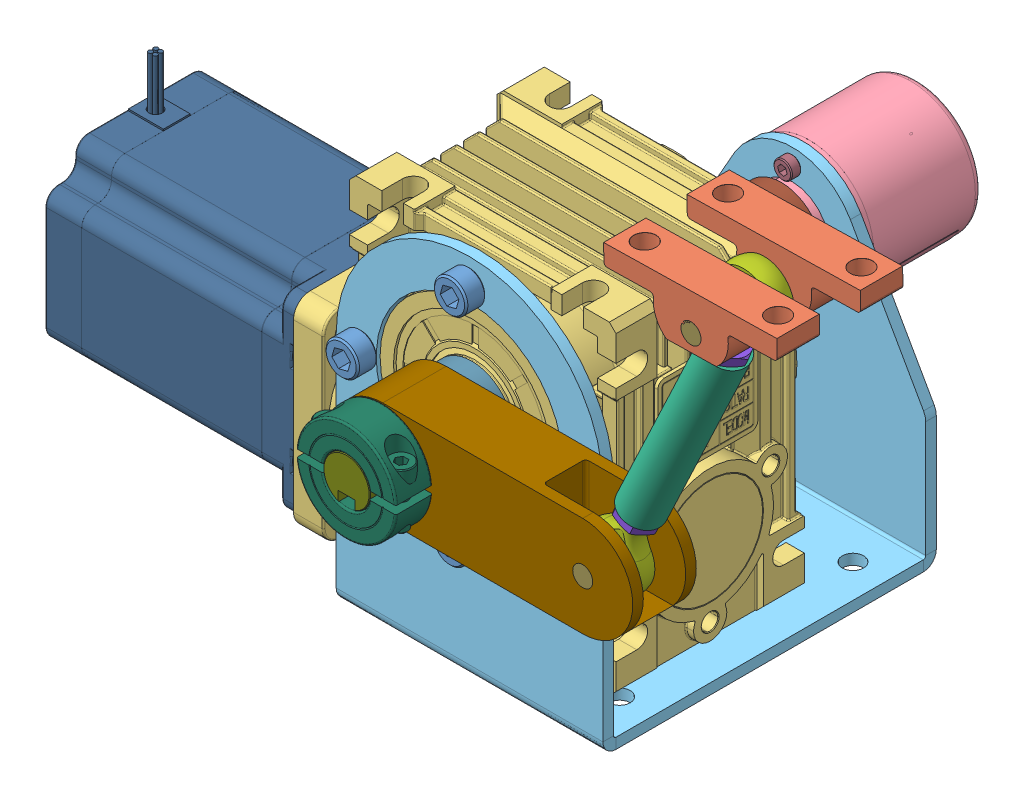
SolidWorks assembly base_motor_linkage_assembly, configuration Default. Lengths in mm.
Overall size (258.89 171.3 171.48).
30 component instances, 17 part files, 54 mates.
Components (placement in the parent):
- 91292A135_M6x16mm_stainless_steel_socket_head_screw-4: 91292A135_M6x16mm_stainless_steel_socket_head_screw [91292A135] at (-204.1211 102.5 84) x (0.718986 0.695024 0) z (0 0 -1) size (10 10 22)
- base_linkage_mounting_block-1: base_linkage_mounting_block [Default] at (-102.5488 169.6402 135.375) x (-0.999802 -0.019915 0) z (0 0 1) size (52 16 12.7)
- NMRV30_nema_23_worm_gearbox-1: NMRV30_nema_23_worm_gearbox [Default] at (-204.1211 70 67.825) x (0 0 -1) z (-1 0 0) size (63.01 100 95.01)
- base_linkage_mounting_block-2: base_linkage_mounting_block [Default] at (-102.5488 169.6402 110.375) x (-0.999802 -0.019915 0) z (0 0 1) size (52 16 12.7)
- base_encoder-1: base_encoder [Default] at (-204.1211 70 -34.4) x (0 -1 0) z (0 0 1) size (38.8 41.72 51.3)
- base_motor_mount-1: base_motor_mount [Default] at (-204.1211 0 50) x (0 0 1) z (-1 0 0) size (100 110 80)
- base_linkage_assembly-1: base_linkage_assembly [Default] at (-117.3362 146.1206 96.5987) x (0.904512 -0.426442 -0.002247) z (-0.426443 -0.904514 0) size (19.02 15.01 117)
  - base_linkage-1: base_linkage [Default] at (8.1889 19.9448 61.2744) size (12 12 60)
  - 59935K82_M6_ball_joint_rod_end-1: 59935K82_M6_ball_joint_rod_end [59935K82] at (8.1889 19.9448 66.2744) x (0.999997 0.002247 0) z (0.002247 -0.999997 0) size (19 45.5 9)
  - 59935K82_M6_ball_joint_rod_end-2: 59935K82_M6_ball_joint_rod_end [59935K82] at (8.1889 19.9448 -3.7256) x (-0.999997 -0.002247 0) z (0.002247 -0.999997 0) size (19 45.5 9)
  - 94168A113_M6_steel_hex_jam_nut-1: 94168A113_M6_steel_hex_jam_nut [94168A113] at (8.1889 19.9448 62.8744) x (0.8649 0.501945 0) z (0 0 1) size (10 11.55 3.2)
  - 94168A113_M6_steel_hex_jam_nut-2: 94168A113_M6_steel_hex_jam_nut [94168A113] at (8.1889 19.9448 -0.3256) x (0.8649 0.501945 0) z (0 0 1) size (10 11.55 3.2)
- base_cam-1: base_cam [Default] at (-204.1211 70 126.05) x (-1 0 0) z (0 1 0) size (90 19.05 30)
- 23HS30-2804S_nema_23_stepper_motor-1: 23HS30-2804S_nema_23_stepper_motor [Default] at (-335.1211 40 67.825) x (0 0 1) z (1 0 0) size (57.02 72.51 97)
- base_encoder_shaft_coupling-1: base_encoder_shaft_coupling [Default] at (-204.1211 70 6.5) x (0.993457 0.114205 0) z (0.114205 -0.993457 0) size (25 25 25)
- 4634T323_6mm_aluminum_shaft-1: 4634T323_6mm_aluminum_shaft [4634T323] at (-102.3297 158.6424 107.2) x (-0.999287 0.037752 0) z (0 0 1) size (6 6 19.05)
- 4634T323_6mm_aluminum_shaft-2: 4634T323_6mm_aluminum_shaft [4634T323] at (-102.3297 158.6424 125.85) x (-0.999287 0.037752 0) z (0 0 1) size (6 6 19.05)
- 90348A005_M3x8mm_stainless_steel_socket_head_screw-1: 90348A005_M3x8mm_stainless_steel_socket_head_screw [90348A005] at (-204.1211 85.5 -4.825) x (-0.948512 -0.316742 0) z (0 0 -1) size (5.5 5.5 11)
- base_motor_shaft_spacer-1: base_motor_shaft_spacer [Default] at (-204.1211 70 106.825) x (0.999152 -0.041181 0) z (0.041181 0.999152 0) size (25 7.5 25)
- 6063K32_14mm_shaft_collar-1: 6063K32_14mm_shaft_collar [6063K32] at (-204.1211 70 131.55) x (-1 0 0) z (0 0 -1) size (29.97 30 11.06)
- 1439K26_14mm_keyed_shaft-1: 1439K26_14mm_keyed_shaft [1439K26] at (-204.1211 70 76.9) x (-1 0 0) z (0 0 1) size (14 13.54 120)
- 92288A725_5mmx5mm_machine_key_stock-1: 92288A725_5mmx5mm_machine_key_stock [92288A725] at (-204.1211 63.2 232.775) size (5 5 19.05)
- 92288A725_5mmx5mm_machine_key_stock-2: 92288A725_5mmx5mm_machine_key_stock [92288A725] at (-204.1211 63.2 259.5) size (5 5 19.05)
- 92288A725_5mmx5mm_machine_key_stock-3: 92288A725_5mmx5mm_machine_key_stock [92288A725] at (-204.1211 63.2 188.825) size (5 5 19.05)
- 4634T323_6mm_aluminum_shaft-3: 4634T323_6mm_aluminum_shaft [4634T323] at (-144.1211 70 116.525) x (-0.999287 0.037752 0) z (0 0 1) size (6 6 19.05)
- 90348A005_M3x8mm_stainless_steel_socket_head_screw-2: 90348A005_M3x8mm_stainless_steel_socket_head_screw [90348A005] at (-217.1115 63 -4.825) x (-0.948512 -0.316742 0) z (0 0 -1) size (5.5 5.5 11)
- 90348A005_M3x8mm_stainless_steel_socket_head_screw-3: 90348A005_M3x8mm_stainless_steel_socket_head_screw [90348A005] at (-191.1308 63 -4.825) x (-0.948512 -0.316742 0) z (0 0 -1) size (5.5 5.5 11)
- 91292A135_M6x16mm_stainless_steel_socket_head_screw-5: 91292A135_M6x16mm_stainless_steel_socket_head_screw [91292A135] at (-236.6211 70 84) x (0.718986 0.695024 0) z (0 0 -1) size (10 10 22)
- 91292A135_M6x16mm_stainless_steel_socket_head_screw-6: 91292A135_M6x16mm_stainless_steel_socket_head_screw [91292A135] at (-171.6211 70 84) x (0.718986 0.695024 0) z (0 0 -1) size (10 10 22)
- 91292A135_M6x16mm_stainless_steel_socket_head_screw-7: 91292A135_M6x16mm_stainless_steel_socket_head_screw [91292A135] at (-204.1211 37.5 84) x (0.718986 0.695024 0) z (0 0 -1) size (10 10 22)
Mates (geometry in assembly coordinates):
- Concentric1: concentric anti-aligned: cylinder of base_motor_shaft_spacer-1 through (-204.1211 70 99.325) axis (0 0 1) radius 7; cylinder of 1439K26_14mm_keyed_shaft-1 through (-204.1211 70 136.9) axis (0 0 -1) radius 7
- Width1: width anti-aligned: plane of 4634T323_6mm_aluminum_shaft-3 through (-144.1211 70 126.05) normal (0 0 1); plane of 4634T323_6mm_aluminum_shaft-3 through (-144.1211 70 107) normal (0 0 -1); plane of base_cam-1 through (-204.1211 70 107) normal (0 0 -1); plane of base_cam-1 through (-204.1211 70 126.05) normal (0 0 1)
- Coincident1: coincident anti-aligned: plane of NMRV30_nema_23_worm_gearbox-1 through (-204.1211 70 99.325) normal (0 0 1); plane of base_motor_shaft_spacer-1 through (-204.1211 70 99.325) normal (0 0 -1)
- Concentric2: concentric anti-aligned: cylinder of base_cam-1 through (-144.1211 70 107) axis (0 0 1) radius 2.995; cylinder of 4634T323_6mm_aluminum_shaft-3 through (-144.1211 70 126.05) axis (0 0 -1) radius 3
- Width2: width aligned: plane of 92288A725_5mmx5mm_machine_key_stock-2 through (-204.1211 63.2 126.05) normal (0 0 1); plane of 92288A725_5mmx5mm_machine_key_stock-2 through (-204.1211 63.2 107) normal (0 0 -1); plane of base_cam-1 through (-204.1211 70 126.05) normal (0 0 1); plane of base_cam-1 through (-204.1211 70 107) normal (0 0 -1)
- Coincident2: coincident anti-aligned: plane of base_cam-1 through (-204.1211 70 126.05) normal (0 0 1); plane of 6063K32_14mm_shaft_collar-1 through (-204.1211 70 126.05) normal (0 0 -1)
- Distance1: distance = 1 mm anti-aligned: plane of base_encoder_shaft_coupling-1 through (-204.1211 70 6.5) normal (0 0 -1); plane of base_encoder-1 through (-204.1211 70 5.5) normal (0 0 1)
- Distance2: distance = 25 mm: cylinder of base_linkage_mounting_block-2 through (-122.5448 169.2419 104.025) axis (-0.019915 0.999802 0) radius 3.3; cylinder of base_linkage_mounting_block-1 through (-122.5448 169.2419 129.025) axis (-0.019915 0.999802 0) radius 3.3
- Concentric3: concentric anti-aligned: cylinder of 91292A135_M6x16mm_stainless_steel_socket_head_screw-4 through (-204.1211 102.5 100) axis (0 0 -1) radius 3; cylinder of base_motor_mount-1 through (-204.1211 102.5 100) axis (0 0 1) radius 3.2
- Distance3: distance = 7 mm anti-aligned: plane of base_motor_mount-1 through (-204.1211 0 100) normal (0 0 1); plane of base_cam-1 through (-204.1211 70 107) normal (0 0 -1)
- Coincident3: coincident anti-aligned: plane of NMRV30_nema_23_worm_gearbox-1 through (-204.1211 70 96.825) normal (0 0 1); plane of base_motor_mount-1 through (-204.1211 0 96.825) normal (0 0 -1)
- Concentric4: concentric anti-aligned: cylinder of NMRV30_nema_23_worm_gearbox-1 through (-204.1211 70 99.325) axis (0 0 -1) radius 7; cylinder of base_encoder-1 through (-204.1211 70 0) axis (0 0 1) radius 3
- Parallel1: parallel aligned: plane of NMRV30_nema_23_worm_gearbox-1 through (-259.1211 10 97.825) normal (0 -1 0); plane of 23HS30-2804S_nema_23_stepper_motor-1 through (-259.1211 11.5 96.325) normal (0 -1 0)
- Coincident4: coincident anti-aligned: plane of NMRV30_nema_23_worm_gearbox-1 through (-259.1211 70 67.825) normal (-1 0 0); plane of 23HS30-2804S_nema_23_stepper_motor-1 through (-259.1211 40 67.825) normal (1 0 0)
- Parallel2: parallel aligned: plane of NMRV30_nema_23_worm_gearbox-1 through (-204.1211 60.7 99.325) normal (0 1 0); plane of base_cam-1 through (-201.6211 60.6917 107) normal (0 1 0)
- Concentric5: concentric anti-aligned: cylinder of NMRV30_nema_23_worm_gearbox-1 through (-204.1211 70 99.325) axis (0 0 -1) radius 7; cylinder of base_motor_mount-1 through (-204.1211 70 -0.001) axis (0 0 1) radius 28
- Concentric6: concentric anti-aligned: cylinder of base_linkage_assembly-1/59935K82_M6_ball_joint_rod_end-1 through (-144.1211 70 121.025) axis (0 0 -1) radius 3; cylinder of base_cam-1 through (-144.1211 70 107) axis (0 0 1) radius 2.995
- Coincident5: coincident aligned: plane of base_linkage_mounting_block-1 through (-128.5436 169.1224 122.675) normal (-0.999802 -0.019915 0); plane of base_linkage_mounting_block-2 through (-128.5436 169.1224 97.675) normal (-0.999802 -0.019915 0)
- Concentric7: concentric anti-aligned: cylinder of NMRV30_nema_23_worm_gearbox-1 through (-204.1211 70 99.325) axis (0 0 -1) radius 7; cylinder of base_cam-1 through (-204.1211 70 107) axis (0 0 1) radius 7
- Coincident6: coincident aligned: plane of base_linkage_mounting_block-1 through (-109.7286 153.494 122.675) normal (0.019915 -0.999802 0); plane of base_linkage_mounting_block-2 through (-109.7286 153.494 97.675) normal (0.019915 -0.999802 0)
- Concentric8: concentric anti-aligned: cylinder of base_encoder-1 through (-204.1211 70 0) axis (0 0 1) radius 3; cylinder of base_encoder_shaft_coupling-1 through (-204.1211 70 31.5) axis (0 0 -1) radius 3
- Width3: width anti-aligned: plane of base_linkage_assembly-1/59935K82_M6_ball_joint_rod_end-1 through (-156.7652 65.4583 119.65) normal (0 0 1); plane of base_linkage_assembly-1/59935K82_M6_ball_joint_rod_end-1 through (-156.7652 65.4583 113.4) normal (0 0 -1); plane of base_cam-1 through (-204.1211 70 107) normal (0 0 -1); plane of base_cam-1 through (-204.1211 70 126.05) normal (0 0 1)
- Parallel3: parallel anti-aligned: plane of NMRV30_nema_23_worm_gearbox-1 through (-244.1211 13 21.7074) normal (0 -1 0); plane of base_motor_mount-1 through (-204.1211 3.175 50) normal (0 1 0)
- Parallel4: parallel aligned: plane of base_encoder-1 through (-206.5211 71.8 16.9) normal (-1 0 0); plane of base_motor_mount-1 through (-202.5211 85.5 100.001) normal (-1 0 0)
- Concentric9: concentric anti-aligned: cylinder of NMRV30_nema_23_worm_gearbox-1 through (-230.6211 40 67.825) axis (-1 0 0) radius 4.5; cylinder of 23HS30-2804S_nema_23_stepper_motor-1 through (-259.1211 40 67.825) axis (1 0 0) radius 3.175
- Width4: width anti-aligned: plane of base_linkage_mounting_block-2 through (-101.1412 161.4685 110.375) normal (0 0 1); plane of base_linkage_mounting_block-1 through (-101.1412 161.4685 122.675) normal (0 0 -1); plane of base_linkage_assembly-1/59935K82_M6_ball_joint_rod_end-2 through (-89.6856 163.1841 113.4) normal (0 0 -1); plane of base_linkage_assembly-1/59935K82_M6_ball_joint_rod_end-2 through (-89.6856 163.1841 119.65) normal (0 0 1)
- Concentric10: concentric anti-aligned: cylinder of base_linkage_mounting_block-1 through (-102.3297 158.6424 135.375) axis (0 0 1) radius 2.5; cylinder of base_linkage_assembly-1/59935K82_M6_ball_joint_rod_end-2 through (-102.3297 158.6424 121.025) axis (0 0 -1) radius 3
- Coincident7: coincident anti-aligned: plane of base_encoder-1 through (-204.1211 70 0) normal (0 0 1); plane of base_motor_mount-1 through (-204.1211 0 0) normal (0 0 -1)
- Concentric11: concentric aligned: cylinder of base_motor_mount-1 through (-191.1308 63 100.001) axis (0 0 -1) radius 1.6; cylinder of 90348A005_M3x8mm_stainless_steel_socket_head_screw-3 through (-191.1308 63 3.175) axis (0 0 -1) radius 1.5
- Concentric12: concentric aligned: cylinder of 4634T323_6mm_aluminum_shaft-1 through (-102.3297 158.6424 116.725) axis (0 0 -1) radius 3; cylinder of 4634T323_6mm_aluminum_shaft-2 through (-102.3297 158.6424 135.375) axis (0 0 -1) radius 3
- Coincident8: coincident aligned: plane of base_linkage_mounting_block-1 through (-101.1412 161.4685 135.375) normal (0 0 1); plane of 4634T323_6mm_aluminum_shaft-2 through (-102.3297 158.6424 135.375) normal (0 0 1)
- Concentric13: concentric aligned: cylinder of base_motor_mount-1 through (-217.1115 63 100.001) axis (0 0 -1) radius 1.6; cylinder of 90348A005_M3x8mm_stainless_steel_socket_head_screw-2 through (-217.1115 63 3.175) axis (0 0 -1) radius 1.5
- Coincident9: coincident anti-aligned: plane of base_motor_mount-1 through (-204.1211 0 3.175) normal (0 0 1); plane of 90348A005_M3x8mm_stainless_steel_socket_head_screw-1 through (-204.1211 85.5 3.175) normal (0 0 -1)
- Concentric14: concentric aligned: cylinder of NMRV30_nema_23_worm_gearbox-1 through (-204.1211 70 99.325) axis (0 0 -1) radius 7; cylinder of 1439K26_14mm_keyed_shaft-1 through (-204.1211 70 136.9) axis (0 0 -1) radius 7
- Coincident10: coincident anti-aligned: plane of base_encoder-1 through (-204.1211 70 16.9) normal (0 0 1); plane of 1439K26_14mm_keyed_shaft-1 through (-204.1211 70 16.9) normal (0 0 -1)
- Concentric15: concentric anti-aligned: cylinder of base_linkage_mounting_block-2 through (-102.3297 158.6424 110.375) axis (0 0 1) radius 2.5; cylinder of 4634T323_6mm_aluminum_shaft-1 through (-102.3297 158.6424 116.725) axis (0 0 -1) radius 3
- Coincident11: coincident aligned: plane of 90348A005_M3x8mm_stainless_steel_socket_head_screw-2 through (-217.1115 63 6.175) normal (0 0 1); plane of 90348A005_M3x8mm_stainless_steel_socket_head_screw-3 through (-191.1308 63 6.175) normal (0 0 1)
- Concentric16: concentric aligned: cylinder of base_motor_mount-1 through (-204.1211 85.5 100.001) axis (0 0 -1) radius 1.6; cylinder of 90348A005_M3x8mm_stainless_steel_socket_head_screw-1 through (-204.1211 85.5 3.175) axis (0 0 -1) radius 1.5
- Coincident12: coincident aligned: plane of 90348A005_M3x8mm_stainless_steel_socket_head_screw-1 through (-204.1211 85.5 6.175) normal (0 0 1); plane of 90348A005_M3x8mm_stainless_steel_socket_head_screw-2 through (-217.1115 63 6.175) normal (0 0 1)
- Width5: width anti-aligned: plane of 92288A725_5mmx5mm_machine_key_stock-3 through (-206.6211 60.7 341.325) normal (-1 0 0); plane of 92288A725_5mmx5mm_machine_key_stock-3 through (-201.6211 60.7 341.325) normal (1 0 0); plane of NMRV30_nema_23_worm_gearbox-1 through (-206.6211 70 99.325) normal (1 0 0); plane of NMRV30_nema_23_worm_gearbox-1 through (-201.6211 70 99.325) normal (-1 0 0)
- Coincident13: coincident anti-aligned: plane of NMRV30_nema_23_worm_gearbox-1 through (-204.1211 60.7 99.325) normal (0 1 0); plane of 92288A725_5mmx5mm_machine_key_stock-3 through (-201.6211 60.7 341.325) normal (0 -1 0)
- Coincident14: coincident aligned: plane of NMRV30_nema_23_worm_gearbox-1 through (-204.1211 70 36.325) normal (0 0 -1); plane of 92288A725_5mmx5mm_machine_key_stock-3 through (-204.1211 63.2 36.325) normal (0 0 -1)
- Coincident15: coincident aligned: plane of NMRV30_nema_23_worm_gearbox-1 through (-204.1211 70 99.325) normal (0 0 1); plane of 92288A725_5mmx5mm_machine_key_stock-1 through (-204.1211 63.2 99.325) normal (0 0 1)
- Coincident16: coincident anti-aligned: plane of 91292A135_M6x16mm_stainless_steel_socket_head_screw-4 through (-204.1211 102.5 100) normal (0 0 -1); plane of base_motor_mount-1 through (-204.1211 0 100) normal (0 0 1)
- Coincident17: coincident aligned: plane of base_linkage_mounting_block-2 through (-101.1412 161.4685 97.675) normal (0 0 -1); plane of 4634T323_6mm_aluminum_shaft-1 through (-102.3297 158.6424 97.675) normal (0 0 -1)
- Parallel5: parallel aligned: plane of base_cam-1 through (-144.1211 85 107) normal (0 1 0); plane of 6063K32_14mm_shaft_collar-1 through (-211.0175 68.8 126.05) normal (0 1 0)
- Concentric17: concentric anti-aligned: cylinder of 6063K32_14mm_shaft_collar-1 through (-204.1211 70 126.05) axis (0 0 1) radius 7; cylinder of 1439K26_14mm_keyed_shaft-1 through (-204.1211 70 136.9) axis (0 0 -1) radius 7
- Parallel6: parallel anti-aligned: plane of 1439K26_14mm_keyed_shaft-1 through (-206.6211 66.4617 136.9) normal (0 -1 0); plane of 92288A725_5mmx5mm_machine_key_stock-3 through (-201.6211 65.7 341.325) normal (0 1 0)
- Coincident18: coincident aligned: plane of 92288A725_5mmx5mm_machine_key_stock-2 through (-201.6211 60.7 412) normal (1 0 0); plane of 92288A725_5mmx5mm_machine_key_stock-3 through (-201.6211 60.7 341.325) normal (1 0 0)
- Coincident19: coincident aligned: plane of 92288A725_5mmx5mm_machine_key_stock-1 through (-201.6211 65.7 385.275) normal (0 1 0); plane of 92288A725_5mmx5mm_machine_key_stock-2 through (-201.6211 65.7 412) normal (0 1 0)
- Coincident20: coincident aligned: plane of 92288A725_5mmx5mm_machine_key_stock-2 through (-201.6211 65.7 412) normal (0 1 0); plane of 92288A725_5mmx5mm_machine_key_stock-3 through (-201.6211 65.7 341.325) normal (0 1 0)
- Coincident21: coincident aligned: plane of 92288A725_5mmx5mm_machine_key_stock-1 through (-201.6211 60.7 385.275) normal (1 0 0); plane of 92288A725_5mmx5mm_machine_key_stock-2 through (-201.6211 60.7 412) normal (1 0 0)
- Coincident22: coincident anti-aligned: plane of base_motor_mount-1 through (-204.1211 0 50) normal (0 -1 0)
- Coincident23: coincident anti-aligned: plane of base_motor_mount-1 through (-204.1211 0 0) normal (0 0 -1)
